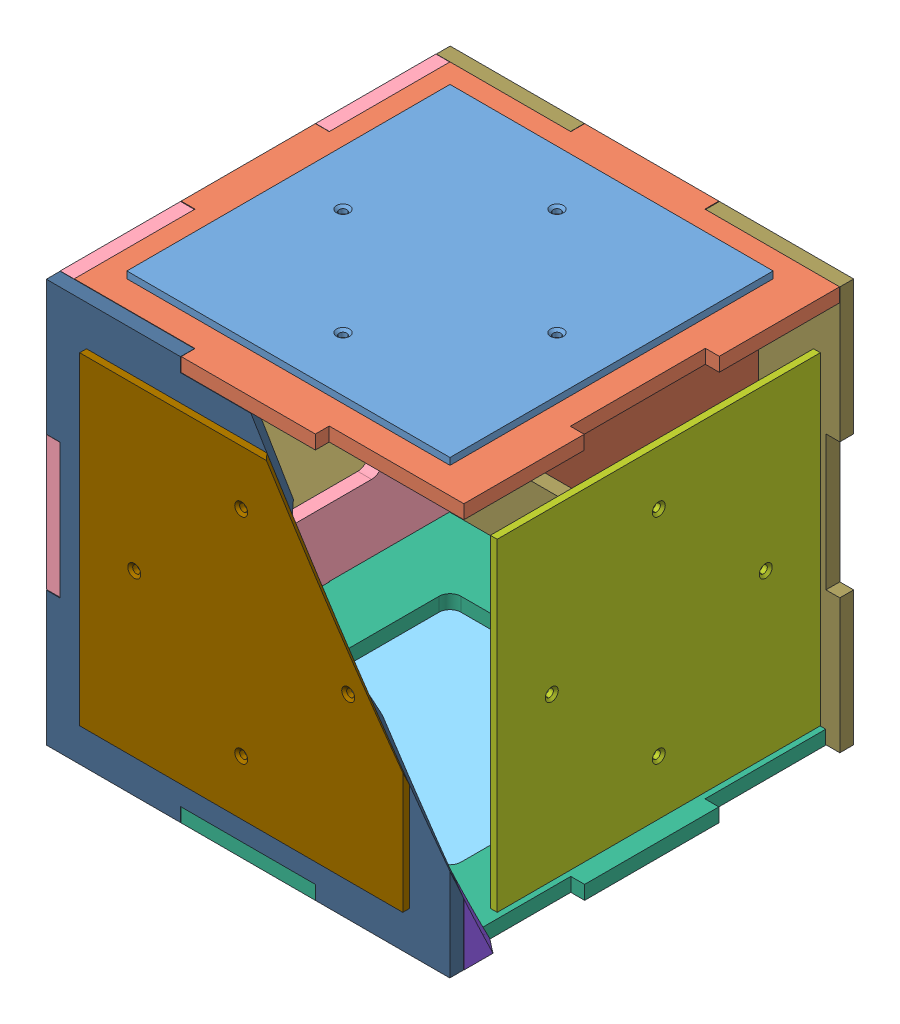
SolidWorks assembly cube_07, configuration cube07. Lengths in mm.
Overall size (97.16 97.16 101.06).
12 component instances, 12 part files, 6 mates.
Components (placement in the parent):
- panel_R^cube_07-13: panel_R^cube_07 [cube01] x (-1 0 0) z (0 0 1) (virtual)
- acrylic_R^cube_07-1: acrylic_R^cube_07 [A] at origin (virtual)
- panel_O^cube_07-8: panel_O^cube_07 [cube01] x (0 -1 0) z (0 0 1) (virtual)
- acrylic_O^cube_07-23: acrylic_O^cube_07 [A] x (0 1 0) z (0 0 1) (virtual)
- panel_Y^cube_07-9: panel_Y^cube_07 [cube01] at origin (virtual)
- acrylic_Y^cube_07-24: acrylic_Y^cube_07 [A] x (-1 0 0) z (0 0 1) (virtual)
- panel_G^cube_07-10: panel_G^cube_07 [cube01] x (0 1 0) z (0 0 1) (virtual)
- acrylic_G^cube_07-25: acrylic_G^cube_07 [A] x (0 -1 0) z (0 0 1) (virtual)
- panel_C^cube_07-11: panel_C^cube_07 [cube01] x (-1 0 0) z (0 -1 0) (virtual)
- acrylic_C^cube_07-26: acrylic_C^cube_07 [B] x (1 0 0) z (0 -1 0) (virtual)
- panel_B^cube_07-13: panel_B^cube_07 [cube01] x (-1 0 0) z (0 1 0) (virtual)
- acrylic_B^cube_07-27: acrylic_B^cube_07 [B] x (1 0 0) z (0 1 0) (virtual)
Mates (geometry in assembly coordinates):
- Coincident1: coincident aligned: plane of panel_R^cube_07-13 through (0 0 0) normal (0 0 1); plane of assembly through (0 0 0) normal (0 0 1)
- Coincident2: coincident anti-aligned: plane of panel_R^cube_07-13; plane of assembly through (0 0 0) normal (1 0 0)
- Coincident3: coincident anti-aligned: plane of panel_R^cube_07-13; plane of assembly through (0 0 0) normal (0 1 0)
- Coincident4: coincident aligned: plane of acrylic_R^cube_07-1 through (0 0 0) normal (0 0 1); plane of assembly through (0 0 0) normal (0 0 1)
- Coincident5: coincident aligned: plane of acrylic_R^cube_07-1 through (0 0 0) normal (1 0 0); plane of assembly through (0 0 0) normal (1 0 0)
- Coincident6: coincident aligned: plane of ? through (0 0 0) normal (0 1 0); plane of assembly through (0 0 0) normal (0 1 0)
